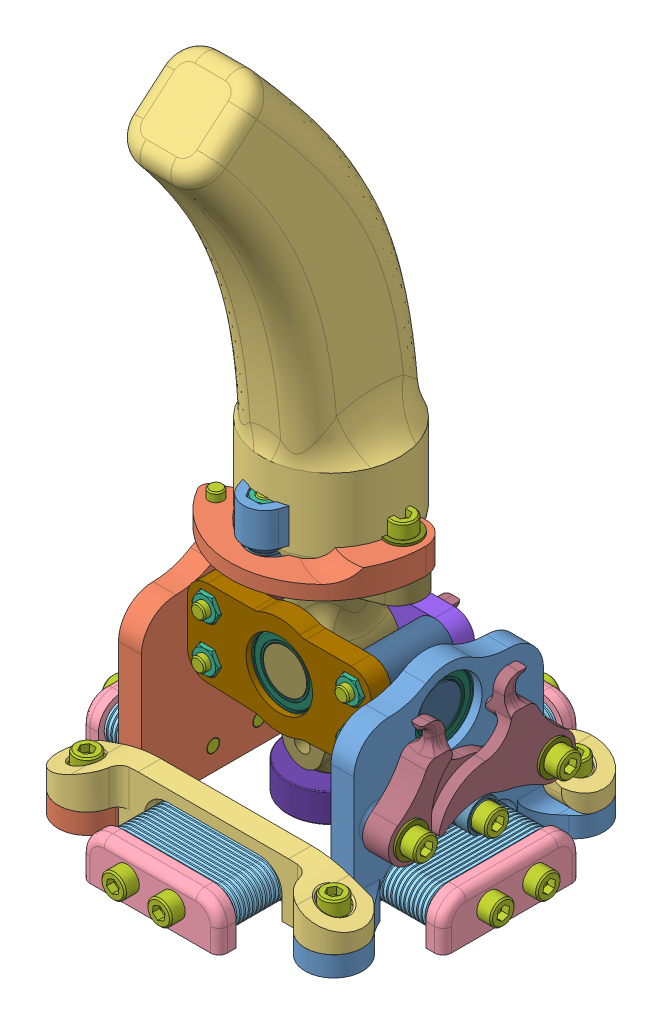
SolidWorks assembly Joystick, configuration Static. Lengths in mm.
Overall size (136 246.22 137.02).
88 component instances, 21 part files, 15 mates.
Components (placement in the parent):
- Base Assembly-1: Base Assembly [Default] at origin size (136 66 136)
  - gimbal_frame_cam_side-1: gimbal_frame_cam_side [Default] at (33 51 0) x (0 0 -1) z (1 0 0) size (104 66 20)
  - gimbal_frame_pot_side_v2-1: gimbal_frame_pot_side_v2 [Default] at (-33 51 0) x (0 0 1) z (-1 0 0) size (104 66 20)
  - mig_mag_footer-1: mig_mag_footer [Default] at (0 10 37) x (-1 0 0) z (0 0 -1) size (106 20 19)
  - mig_mag_footer-2: mig_mag_footer [Default] at (0 10 -37) size (106 20 19)
  - mag cover-1: mag cover [Default] at (57 8 0) size (6 16 48)
  - electromagnet coil-1: electromagnet coil [Default] at (46 8 0) size (21 13 45)
  - hex nut style 1_am-1: hex nut style 1_am [B18.2.4.1M - Hex nut, Style 1,  M5 x 0.8 --D-N] at (33.3 31 25) x (0 0.5 0.866025) z (-1 0 0) size (8 9.24 4.7)
  - hex nut style 1_am-2: hex nut style 1_am [B18.2.4.1M - Hex nut, Style 1,  M5 x 0.8 --D-N] at (33.3 31 -25) x (0 -0.5 0.866025) z (-1 0 0) size (8 9.24 4.7)
  - socket head cap screw_am-14: socket head cap screw_am [B18.3.1M - 5 x 0.8 x 30 Hex SHCS -- 22NHX] at (68 8 -8) x (-1 0 0) z (0 0.924225 0.381849) size (35 8.5 8.5)
  - socket head cap screw_am-15: socket head cap screw_am [B18.3.1M - 5 x 0.8 x 30 Hex SHCS -- 22NHX] at (68 8 8) x (-1 0 0) z (0 0.924225 0.381849) size (35 8.5 8.5)
  - socket head cap screw_am-16: socket head cap screw_am [B18.3.1M - 5 x 0.8 x 30 Hex SHCS -- 22NHX] at (8 8 68) x (0 0 -1) z (-0.381849 0.924225 0) size (35 8.5 8.5)
  - socket head cap screw_am-17: socket head cap screw_am [B18.3.1M - 5 x 0.8 x 30 Hex SHCS -- 22NHX] at (-68 8 8) x (1 0 0) z (0 0.924225 -0.381849) size (35 8.5 8.5)
  - socket head cap screw_am-18: socket head cap screw_am [B18.3.1M - 5 x 0.8 x 30 Hex SHCS -- 22NHX] at (-8 8 -68) x (0 0 1) z (0.381849 0.924225 0) size (35 8.5 8.5)
  - socket head cap screw_am-19: socket head cap screw_am [B18.3.1M - 5 x 0.8 x 30 Hex SHCS -- 22NHX] at (-8 8 68) x (0 0 -1) z (-0.381849 0.924225 0) size (35 8.5 8.5)
  - socket head cap screw_am-20: socket head cap screw_am [B18.3.1M - 5 x 0.8 x 30 Hex SHCS -- 22NHX] at (-68 8 -8) x (1 0 0) z (0 0.924225 -0.381849) size (35 8.5 8.5)
  - socket head cap screw_am-21: socket head cap screw_am [B18.3.1M - 5 x 0.8 x 30 Hex SHCS -- 22NHX] at (8 8 -68) x (0 0 1) z (0.381849 0.924225 0) size (35 8.5 8.5)
  - mag cover-5: mag cover [Default] at (0 8 57) x (0 0 1) z (-1 0 0) size (6 16 48)
  - mag cover-6: mag cover [Default] at (-57 8 0) x (-1 0 0) z (0 0 -1) size (6 16 48)
  - mag cover-7: mag cover [Default] at (0 8 -57) x (0 0 -1) z (1 0 0) size (6 16 48)
  - electromagnet coil-5: electromagnet coil [Default] at (0 8 46) x (0 0 1) z (-1 0 0) size (21 13 45)
  - electromagnet coil-6: electromagnet coil [Default] at (-46 8 0) x (-1 0 0) z (0 0 -1) size (21 13 45)
  - electromagnet coil-7: electromagnet coil [Default] at (0 8 -46) x (0 0 -1) z (1 0 0) size (21 13 45)
  - socket head cap screw_am-22: socket head cap screw_am [B18.3.1M - 5 x 0.8 x 12 Hex SHCS -- 12NHX] at (43 19.04 -42) x (0 -1 0) z (0 0 1) size (17 8.5 8.5)
  - socket head cap screw_am-23: socket head cap screw_am [B18.3.1M - 5 x 0.8 x 12 Hex SHCS -- 12NHX] at (-43 19.04 -42) x (0 -1 0) z (0 0 1) size (17 8.5 8.5)
  - socket head cap screw_am-24: socket head cap screw_am [B18.3.1M - 5 x 0.8 x 12 Hex SHCS -- 12NHX] at (-43 19.04 42) x (0 -1 0) z (0 0 1) size (17 8.5 8.5)
  - socket head cap screw_am-25: socket head cap screw_am [B18.3.1M - 5 x 0.8 x 12 Hex SHCS -- 12NHX] at (43 19.04 42) x (0 -1 0) z (0 0 1) size (17 8.5 8.5)
- Axis Assembly-1: Axis Assembly [Default] at (18 51 0) size (96.4 123.21 70.4) (flexible)
  - gimbal_core_bearing_carrier_non_pot_side-1: gimbal_core_bearing_carrier_non_pot_side [Default] at (-18 0 -14.5) x (-1 0 0) z (0 0 -1) size (64 44 7.5)
  - gimbal_core_bearing_carrier_pot_side-1: gimbal_core_bearing_carrier_pot_side [Default] at (-18 0 14.5) size (64 34.5 7)
  - gimbal_core_non_pot_side-1: gimbal_core_non_pot_side [Default] x (0 0 -1) z (1 0 0) size (24.58 47 25)
  - gimbal_core_pot_side-1: gimbal_core_pot_side [Default] at (-43 0 0) x (0 0 1) z (-1 0 0) size (22 30 20)
  - gimbal_lever_arm-1: gimbal_lever_arm [Default] at (-18 0 0) x (1 0 0) z (0 0 -1) size (57.72 104.81 36)
  - gimbal_cam-1: gimbal_cam [Default] at (25.5 -20 25) x (0 0.02008 -0.999798) z (1 0 0) size (47.46 36.5 9.63)
  - gimbal_cam-2: gimbal_cam [Default] at (34.6 -20 -25) x (0 0.02008 0.999798) z (-1 0 0) size (47.46 36.5 9.63)
  - gimbal_cam-3: gimbal_cam [Default] at (7 -20 -20.5) x (-0.999798 0.02008 0) z (0 0 -1) size (47.46 36.5 9.63)
  - gimbal_cam-4: gimbal_cam [Default] at (-43 -20 -29.6) x (0.999798 0.02008 0) z (0 0 1) size (47.46 36.5 9.63)
  - 685 Bearing-1: 685 Bearing [Default] at (-18 -25 -27.6) x (-0.212055 -0.977258 0) z (0 0 1) size (11 11 5)
  - 685 Bearing-2: 685 Bearing [Default] at (-18 -25 -22.5) x (0.074604 0.997213 0) z (0 0 1) size (11 11 5)
  - 685 Bearing-3: 685 Bearing [Default] at (27.5 -25 0) x (0 0.009189 -0.999958) z (1 0 0) size (11 11 5)
  - 685 Bearing-4: 685 Bearing [Default] at (32.6 -25 0) x (0 0.988805 -0.149215) z (1 0 0) size (11 11 5)
  - 6802 Bearing-1: 6802 Bearing [Default] at (-53.5 0 0) x (1 0 0) z (0 0.012241 0.999925) size (5 24 24)
  - 6802 Bearing-2: 6802 Bearing [Default] at (17.5 0 0) x (1 0 0) z (0 -0.040824 0.999166) size (5 24 24)
  - 6802 Bearing-3: 6802 Bearing [Default] at (-18 0 -13.5) x (0 0 1) z (-0.979067 0.203538 0) size (5 24 24)
  - 6802 Bearing-4: 6802 Bearing [Default] at (-18 0 13.5) x (0 0 -1) z (0.872831 -0.488023 0) size (5 24 24)
  - MF105 Bearing-1: MF105 Bearing [Default] at (-43 -20 -28.4) size (11.6 11.6 4)
  - MF105 Bearing-2: MF105 Bearing [Default] at (-43 -20 -21.8) x (-0.910921 -0.412581 0) z (0 0 -1) size (11.6 11.6 4)
  - MF105 Bearing-3: MF105 Bearing [Default] at (7 -20 -28.3) x (0.979695 0.200494 0) z (0 0 1) size (11.6 11.6 4)
  - MF105 Bearing-4: MF105 Bearing [Default] at (7 -20 -21.7) x (-0.975001 0.222199 0) z (0 0 -1) size (11.6 11.6 4)
  - MF105 Bearing-5: MF105 Bearing [Default] at (33.3 -20 25) x (0 0.012241 0.999925) z (-1 0 0) size (11.6 11.6 4)
  - MF105 Bearing-6: MF105 Bearing [Default] at (26.7 -20 25) x (0 -0.012241 -0.999925) z (1 0 0) size (11.6 11.6 4)
  - MF105 Bearing-7: MF105 Bearing [Default] at (26.8 -20 -25) x (0 -0.012241 -0.999925) z (1 0 0) size (11.6 11.6 4)
  - MF105 Bearing-8: MF105 Bearing [Default] at (33.4 -20 -25) x (0 0.012241 0.999925) z (-1 0 0) size (11.6 11.6 4)
  - Magnetic Core-1: Magnetic Core [Default] at (-18 -43.81 0) x (0.994167 0 0.107854) z (-0.107854 0 0.994167) size (30 10 30)
  - flat washer narrow_am-2: flat washer narrow_am [B18.22M - Plain washer, 5 mm, narrow] at (-18 -43.81 0) x (0 1 0) z (0.053545 0 0.998565) size (1.4 11 11)
  - socket head cap screw_am-1: socket head cap screw_am [B18.3.1M - 5 x 0.8 x 16 Hex SHCS -- 16NHX] at (-18 -50.21 0) x (0 1 0) z (0.054252 0 0.998527) size (21 8.5 8.5)
  - socket head cap screw_am-2: socket head cap screw_am [B18.3.1M - 5 x 0.8 x 35 Hex SHCS -- 22NHX] at (-43 8 -18.5) x (0 0 1) z (-0.998547 -0.053886 0) size (40 8.5 8.5)
  - socket head cap screw_am-3: socket head cap screw_am [B18.3.1M - 5 x 0.8 x 35 Hex SHCS -- 22NHX] at (-43 -8 -18.5) x (0 0 1) z (-0.998547 -0.053886 0) size (40 8.5 8.5)
  - socket head cap screw_am-4: socket head cap screw_am [B18.3.1M - 5 x 0.8 x 35 Hex SHCS -- 22NHX] at (7 8 -18.5) x (0 0 1) z (-0.998547 -0.053886 0) size (40 8.5 8.5)
  - socket head cap screw_am-5: socket head cap screw_am [B18.3.1M - 5 x 0.8 x 35 Hex SHCS -- 22NHX] at (7 -8 -18.5) x (0 0 1) z (-0.998547 -0.053886 0) size (40 8.5 8.5)
  - socket head cap screw_am-6: socket head cap screw_am [B18.3.1M - 5 x 0.8 x 20 Hex SHCS -- 20NHX] at (-43 -20 -35.4) x (0 0 1) z (-0.998547 -0.053886 0) size (25 8.5 8.5)
  - socket head cap screw_am-7: socket head cap screw_am [B18.3.1M - 5 x 0.8 x 20 Hex SHCS -- 20NHX] at (7 -20 -35.3) x (0 0 1) z (-0.998547 -0.053886 0) size (25 8.5 8.5)
  - socket head cap screw_am-8: socket head cap screw_am [B18.3.1M - 5 x 0.8 x 20 Hex SHCS -- 20NHX] at (40.4 -20 -25) x (-1 0 0) z (0 0.924996 0.379978) size (25 8.5 8.5)
  - socket head cap screw_am-9: socket head cap screw_am [B18.3.1M - 5 x 0.8 x 20 Hex SHCS -- 20NHX] at (40.3 -20 25) x (-1 0 0) z (0 0.924996 0.379978) size (25 8.5 8.5)
  - socket head cap screw_am-12: socket head cap screw_am [B18.3.1M - 5 x 0.8 x 25 Hex SHCS -- 25NHX] at (40.1 -25 0) x (-1 0 0) z (0 0.924996 0.379978) size (30 8.5 8.5)
  - socket head cap screw_am-13: socket head cap screw_am [B18.3.1M - 5 x 0.8 x 25 Hex SHCS -- 25NHX] at (-18 -25 -35.1) x (0 0 1) z (-0.998636 -0.052212 0) size (30 8.5 8.5)
  - hex nut style 1_am-1: hex nut style 1_am [B18.2.4.1M - Hex nut, Style 1,  M5 x 0.8 --D-N] at (7 8 19.2) x (0.866025 -0.5 0) z (0 0 1) size (8 9.24 4.7)
  - hex nut style 1_am-2: hex nut style 1_am [B18.2.4.1M - Hex nut, Style 1,  M5 x 0.8 --D-N] at (7 -8 19.2) x (0.866025 -0.5 0) z (0 0 1) size (8 9.24 4.7)
  - hex nut style 1_am-3: hex nut style 1_am [B18.2.4.1M - Hex nut, Style 1,  M5 x 0.8 --D-N] at (-43 8 19.2) x (0.866025 -0.5 0) z (0 0 1) size (8 9.24 4.7)
  - hex nut style 1_am-4: hex nut style 1_am [B18.2.4.1M - Hex nut, Style 1,  M5 x 0.8 --D-N] at (-43 -8 19.2) x (0.866025 -0.5 0) z (0 0 1) size (8 9.24 4.7)
  - hex nut style 1_am-5: hex nut style 1_am [B18.2.4.1M - Hex nut, Style 1,  M5 x 0.8 --D-N] at (-43 -20 -9.8) x (0.866025 -0.5 0) z (0 0 1) size (8 9.24 4.7)
  - hex nut style 1_am-6: hex nut style 1_am [B18.2.4.1M - Hex nut, Style 1,  M5 x 0.8 --D-N] at (7 -20 -9.8) x (0.866025 -0.5 0) z (0 0 1) size (8 9.24 4.7)
  - hex nut style 1_am-7: hex nut style 1_am [B18.2.4.1M - Hex nut, Style 1,  M5 x 0.8 --D-N] at (10.3 -25 0) x (0 -0.5 0.866025) z (-1 0 0) size (8 9.24 4.7)
  - 6802 Bearing-5: 6802 Bearing [Default] at (-18 40.5 0) x (0 1 0) z (0.996415 0 0.084594) size (5 24 24)
  - 685 Bearing-5: 685 Bearing [Default] at (-18 63.5 0) x (-0.742274 0 -0.670097) z (0 1 0) size (11 11 5)
  - Grip attach-1: Grip attach [Default] at (-18 38 0) x (-1 0 0) z (0 0 -1) size (31.31 35 45.5)
  - 685 Bearing-6: 685 Bearing [Default] at (-18 39.7 23) x (0 0 1) z (0 -1 0) size (11 11 5)
  - socket head cap screw_am-14: socket head cap screw_am [B18.3.1M - 5 x 0.8 x 20 Hex SHCS -- 20NHX] at (-18 32.2 23) x (0 1 0) z (0.892932 0 0.450191) size (25 8.5 8.5)
  - hex nut style 1_am-8: hex nut style 1_am [B18.2.4.1M - Hex nut, Style 1,  M5 x 0.8 --D-N] at (-18 52.2 23) x (0.866025 0 -0.5) z (0 -1 0) size (8 9.24 4.7)
  - gimbal_twist_cam-1: gimbal_twist_cam [Default] at (7 37.2 0) x (-1 0 0) z (0 0 -1) size (61.45 9.74 43)
  - MF105 Bearing-9: MF105 Bearing [Default] at (7 38.4 0) x (0.992202 0 0.124638) z (0 1 0) size (11.6 11.6 4)
  - MF105 Bearing-10: MF105 Bearing [Default] at (7 45 0) x (-0.862572 0 -0.505934) z (0 -1 0) size (11.6 11.6 4)
  - socket head cap screw_am-15: socket head cap screw_am [B18.3.1M - 5 x 0.8 x 20 Hex SHCS -- 20NHX] at (7 52 0) x (0 -1 0) z (-0.051257 0 0.998686) size (25 8.5 8.5)
  - hex nut style 1_am-9: hex nut style 1_am [B18.2.4.1M - Hex nut, Style 1,  M5 x 0.8 --D-N] at (7 27.9 0) x (1 0 0) z (0 -1 0) size (8 9.24 4.7)
  - socket head cap screw_am-16: socket head cap screw_am [B18.3.1M - 5 x 0.8 x 8 Hex SHCS -- 8NHX] at (-40.3698 32.2 17.6716) x (0 1 0) z (0.152957 0 0.988233) size (13 8.5 8.5)
  - socket head cap screw_am-17: socket head cap screw_am [B18.3.1M - 5 x 0.8 x 8 Hex SHCS -- 8NHX] at (-39.2223 41.5 -13.2142) x (0 -1 0) z (0.189446 0 0.981891) size (13 8.5 8.5)
- Grip-1: Grip [Default] at (0 89 0) x (-1 0 0) z (0 0 -1) size (48.12 157.22 103.93)
  - Grip Proxy-1: Grip Proxy [Default] at origin size (48.12 157.22 103.93)
Mates (geometry in assembly coordinates):
- Coincident2: coordinate: point of Base Assembly-1
- Concentric1: concentric aligned: cylinder of Base Assembly-1/gimbal_frame_cam_side-1 through (38.1 51 0) axis (-1 0 0) radius 12.1; cylinder of Axis Assembly-1/gimbal_core_non_pot_side-1 through (38 51 0) axis (-1 0 0) radius 7.3
- Width1: width aligned: plane of Base Assembly-1/gimbal_frame_pot_side_v2-1 through (-33 51 0) normal (1 0 0); plane of Base Assembly-1/gimbal_frame_cam_side-1 through (33 51 0) normal (-1 0 0); plane of Axis Assembly-1/gimbal_core_non_pot_side-1 through (38 51 0) normal (1 0 0); plane of Axis Assembly-1/gimbal_core_pot_side-1 through (-38 51 0) normal (-1 0 0)
- Coincident4: coincident aligned: plane of Axis Assembly-1/gimbal_lever_arm-1 through (0 51 0) normal (1 0 0)
- Coincident5: coincident anti-aligned: plane of Axis Assembly-1/gimbal_lever_arm-1 through (0 51 0) normal (0 0 -1)
- Parallel3: parallel anti-aligned: plane of Axis Assembly-1/Grip attach-1 through (0 89 0) normal (-1 0 0)
- Concentric2: concentric: cylinder of Axis Assembly-1/gimbal_lever_arm-1 through (-21.2223 73.35 -13.2142) axis (0 1 0) radius 2.25; cylinder of socket head cap screw_am-1 through (-21.2223 124.25 -13.2142) axis (0 1 0) radius 4.25
- Coincident6: coincident: plane of Axis Assembly-1/gimbal_lever_arm-1 through (0 87.5 0) normal (0 1 0); plane of socket head cap screw_am-1 through (-16.9723 87.5 -13.2142) normal (0 -1 0)
- Concentric3: concentric aligned: cylinder of Axis Assembly-1/gimbal_lever_arm-1 through (-21.2223 73.35 -13.2142) axis (0 1 0) radius 2.25; cylinder of socket head cap screw_am-3 through (-21.2223 124.25 -13.2142) axis (0 1 0) radius 4.25
- Coincident8: coincident anti-aligned: plane of Axis Assembly-1/gimbal_lever_arm-1 through (0 87.5 0) normal (0 1 0); plane of socket head cap screw_am-3 through (-16.9723 87.5 -13.2142) normal (0 -1 0)
- Parallel4: parallel aligned: plane of Axis Assembly-1 through (18 51 0) normal (0 0 1)
- Parallel5: parallel aligned: plane of Axis Assembly-1 through (18 51 0) normal (1 0 0)
- Concentric4: concentric aligned: cylinder of Axis Assembly-1/Grip attach-1 through (0 124 0) axis (0 -1 0) radius 15; cylinder of Grip-1/Grip Proxy-1 through (0 119.67 0) axis (0 -1 0) radius 24.0598
- Coincident9: coincident aligned: plane of Axis Assembly-1/Grip attach-1 through (0 89 0) normal (0 -1 0); plane of Grip-1/Grip Proxy-1 through (-15.335 89 22) normal (0 -1 0)
- Coincident10: coincident aligned: plane of Axis Assembly-1/Grip attach-1 through (0 89 0) normal (-1 0 0); plane of Grip-1/Grip Proxy-1 through (0 89 0) normal (-1 0 0)
